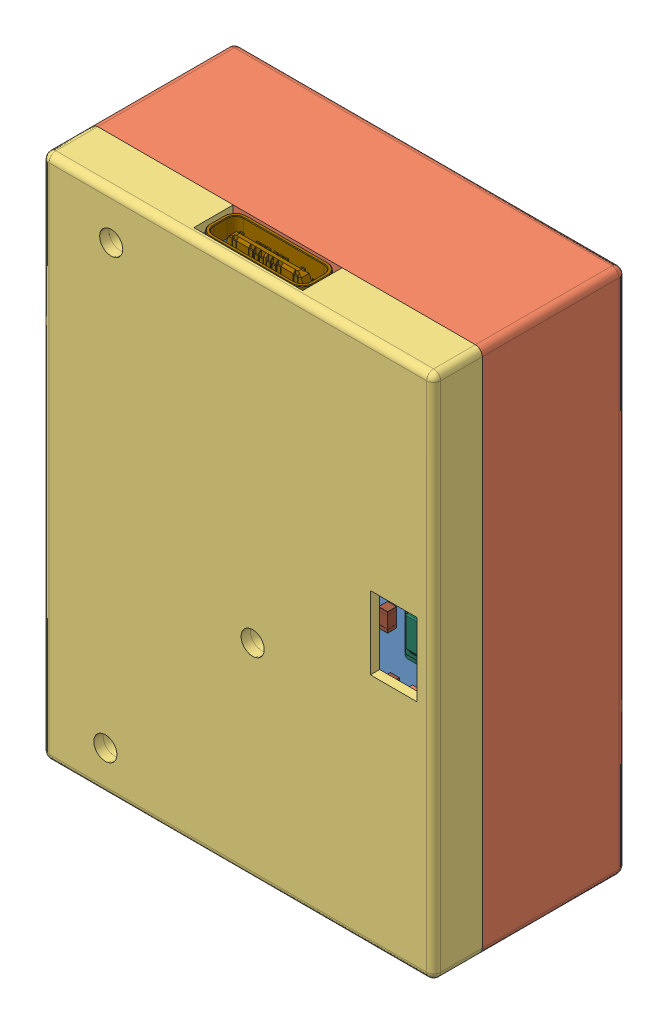
SolidWorks assembly 装配体v3.0, configuration 默认. Lengths in mm.
Overall size (33.77 45.37 16.59).
124 component instances, 21 part files, 8 mates.
Components (placement in the parent):
- 3D_主控_2025-09-16.step-1: 3D_主控_2025-09-16.step [默认] at (-99.2028 -82.7519 -1.9344) size (29.97 44.3 5.71)
  - U3~DFN-4_L1.5-W1.5-P0.8-TL-EP~DFN-4_L1.5-W1.5-P0.8~N7qM.step-1: U3~DFN-4_L1.5-W1.5-P0.8-TL-EP~DFN-4_L1.5-W1.5-P0.8~N7qM.step [默认] at (23.622 -32.2581 0) x (0 -1 0) z (0 0 -1) size (1.52 1.52 0.55)
    - DFN-4_L1.5-W1.5-P0.8-TL-EP~DFN-4_L1.5-W1.5-P0.8~N7qM.step-1: DFN-4_L1.5-W1.5-P0.8-TL-EP~DFN-4_L1.5-W1.5-P0.8~N7qM.step [默认] at origin size (1.52 1.52 0.55)
  - R1~R0603~R0603~N7qM.step-1: R1~R0603~R0603~N7qM.step [默认] at (25.6541 -14.224 1.5862) x (0 1 0) z (0 0 1) size (1.62 0.81 0.45)
    - R0603~R0603~N7qM.step-1: R0603~R0603~N7qM.step [默认] at origin size (1.62 0.81 0.45)
  - R1~R0603~R0603~N7qM.step-2: R1~R0603~R0603~N7qM.step [默认] at (23.241 -17.78 1.5862) size (1.62 0.81 0.45)
    - R0603~R0603~N7qM.step-1: R0603~R0603~N7qM.step [默认] at origin size (1.62 0.81 0.45)
  - R1~R0603~R0603~N7qM.step-3: R1~R0603~R0603~N7qM.step [默认] at (23.495 -34.7981 1.5862) x (0 -1 0) z (0 0 1) size (1.62 0.81 0.45)
    - R0603~R0603~N7qM.step-1: R0603~R0603~N7qM.step [默认] at origin size (1.62 0.81 0.45)
  - R1~R0603~R0603~N7qM.step-4: R1~R0603~R0603~N7qM.step [默认] at (27.5263 -28.0739 1.5862) x (0 1 0) z (0 0 1) size (1.62 0.81 0.45)
    - R0603~R0603~N7qM.step-1: R0603~R0603~N7qM.step [默认] at origin size (1.62 0.81 0.45)
  - R1~R0603~R0603~N7qM.step-5: R1~R0603~R0603~N7qM.step [默认] at (11.684 -10.668 1.5862) x (-1 0 0) z (0 0 1) size (1.62 0.81 0.45)
    - R0603~R0603~N7qM.step-1: R0603~R0603~N7qM.step [默认] at origin size (1.62 0.81 0.45)
  - R1~R0603~R0603~N7qM.step-6: R1~R0603~R0603~N7qM.step [默认] at (11.684 -9.144 1.5862) x (-1 0 0) z (0 0 1) size (1.62 0.81 0.45)
    - R0603~R0603~N7qM.step-1: R0603~R0603~N7qM.step [默认] at origin size (1.62 0.81 0.45)
  - R1~R0603~R0603~N7qM.step-7: R1~R0603~R0603~N7qM.step [默认] at (25.4001 -31.6231 1.5862) x (0 -1 0) z (0 0 1) size (1.62 0.81 0.45)
    - R0603~R0603~N7qM.step-1: R0603~R0603~N7qM.step [默认] at origin size (1.62 0.81 0.45)
  - R1~R0603~R0603~N7qM.step-8: R1~R0603~R0603~N7qM.step [默认] at (3.556 -9.398 1.5862) x (0 -1 0) z (0 0 1) size (1.62 0.81 0.45)
    - R0603~R0603~N7qM.step-1: R0603~R0603~N7qM.step [默认] at origin size (1.62 0.81 0.45)
  - R1~R0603~R0603~N7qM.step-9: R1~R0603~R0603~N7qM.step [默认] at (25.3867 -28.0538 1.5862) x (0 -1 0) z (0 0 1) size (1.62 0.81 0.45)
    - R0603~R0603~N7qM.step-1: R0603~R0603~N7qM.step [默认] at origin size (1.62 0.81 0.45)
  - R1~R0603~R0603~N7qM.step-10: R1~R0603~R0603~N7qM.step [默认] at (2.032 -14.859 1.5862) x (0 -1 0) z (0 0 1) size (1.62 0.81 0.45)
    - R0603~R0603~N7qM.step-1: R0603~R0603~N7qM.step [默认] at origin size (1.62 0.81 0.45)
  - R1~R0603~R0603~N7qM.step-11: R1~R0603~R0603~N7qM.step [默认] at (3.683 -14.859 1.5862) x (0 -1 0) z (0 0 1) size (1.62 0.81 0.45)
    - R0603~R0603~N7qM.step-1: R0603~R0603~N7qM.step [默认] at origin size (1.62 0.81 0.45)
  - R1~R0603~R0603~N7qM.step-12: R1~R0603~R0603~N7qM.step [默认] at (22.606 -5.969 1.5862) size (1.62 0.81 0.45)
    - R0603~R0603~N7qM.step-1: R0603~R0603~N7qM.step [默认] at origin size (1.62 0.81 0.45)
  - R1~R0603~R0603~N7qM.step-13: R1~R0603~R0603~N7qM.step [默认] at (22.606 -7.747 1.5862) size (1.62 0.81 0.45)
    - R0603~R0603~N7qM.step-1: R0603~R0603~N7qM.step [默认] at origin size (1.62 0.81 0.45)
  - R1~R0603~R0603~N7qM.step-14: R1~R0603~R0603~N7qM.step [默认] at (11.684 -13.081 1.5862) size (1.62 0.81 0.45)
    - R0603~R0603~N7qM.step-1: R0603~R0603~N7qM.step [默认] at origin size (1.62 0.81 0.45)
  - R1~R0603~R0603~N7qM.step-15: R1~R0603~R0603~N7qM.step [默认] at (24.384 -37.5921 0) x (-1 0 0) z (0 0 -1) size (1.62 0.81 0.45)
    - R0603~R0603~N7qM.step-1: R0603~R0603~N7qM.step [默认] at origin size (1.62 0.81 0.45)
  - R1~R0603~R0603~N7qM.step-16: R1~R0603~R0603~N7qM.step [默认] at (24.384 -39.4971 0) x (-1 0 0) z (0 0 -1) size (1.62 0.81 0.45)
    - R0603~R0603~N7qM.step-1: R0603~R0603~N7qM.step [默认] at origin size (1.62 0.81 0.45)
  - R1~R0603~R0603~N7qM.step-17: R1~R0603~R0603~N7qM.step [默认] at (5.969 -5.842 1.5862) size (1.62 0.81 0.45)
    - R0603~R0603~N7qM.step-1: R0603~R0603~N7qM.step [默认] at origin size (1.62 0.81 0.45)
  - R1~R0603~R0603~N7qM.step-18: R1~R0603~R0603~N7qM.step [默认] at (18.161 -30.8611 1.5862) x (0 -1 0) z (0 0 1) size (1.62 0.81 0.45)
    - R0603~R0603~N7qM.step-1: R0603~R0603~N7qM.step [默认] at origin size (1.62 0.81 0.45)
  - fin~LED_0603~LED-0603_G~N7qM.step-1: fin~LED_0603~LED-0603_G~N7qM.step [默认] at (26.1621 -7.747 1.5862) size (1.6 0.8 0.6)
    - LED_0603~LED-0603_G~N7qM.step-1: LED_0603~LED-0603_G~N7qM.step [默认] at origin size (1.6 0.8 0.6)
  - L1~L0603~L0603_L1.6-W0.8-H0.5_BEAD~N7qM.step-1: L1~L0603~L0603_L1.6-W0.8-H0.5_BEAD~N7qM.step [默认] at (9.144 -28.5751 1.5862) x (0 1 0) z (0 0 1) size (1.6 0.8 0.5)
    - L0603~L0603_L1.6-W0.8-H0.5_BEAD~N7qM.step-1: L0603~L0603_L1.6-W0.8-H0.5_BEAD~N7qM.step [默认] at origin size (1.6 0.8 0.5)
  - in~LED_0603~LED-0603_R~N7qM.step-1: in~LED_0603~LED-0603_R~N7qM.step [默认] at (27.5591 -31.6231 1.5862) x (0 1 0) z (0 0 1) size (1.49 0.75 0.56)
    - LED_0603~LED-0603_R~N7qM.step-1: LED_0603~LED-0603_R~N7qM.step [默认] at origin size (1.49 0.75 0.56)
  - in~LED_0603~LED-0603_R~N7qM.step-2: in~LED_0603~LED-0603_R~N7qM.step [默认] at (26.1621 -5.969 1.5862) size (1.49 0.75 0.56)
    - LED_0603~LED-0603_R~N7qM.step-1: LED_0603~LED-0603_R~N7qM.step [默认] at origin size (1.49 0.75 0.56)
  - U4~HLGA-10L_LPS22HBTR~HLGA-10L_L2.0-W2.0-H0.8-P0.5-LPS22HBTR~N7qM.step-1: U4~HLGA-10L_LPS22HBTR~HLGA-10L_L2.0-W2.0-H0.8-P0.5-LPS22HBTR~N7qM.step [默认] at (23.495 -28.4481 0) x (0 -1 0) z (0 0 -1) size (2 2 0.8)
    - HLGA-10L_LPS22HBTR~HLGA-10L_L2.0-W2.0-H0.8-P0.5-LPS22HBTR~N7qM.step-1: HLGA-10L_LPS22HBTR~HLGA-10L_L2.0-W2.0-H0.8-P0.5-LPS22HBTR~N7qM.step [默认] at origin size (2 2 0.8)
  - U5~DFN-6_L2.5-W2.5-P0.8-BL-EP~DFN-6_L2.5-W2.5-0.9-P0.8-BL-EP~N7qM.step-1: U5~DFN-6_L2.5-W2.5-P0.8-BL-EP~DFN-6_L2.5-W2.5-0.9-P0.8-BL-EP~N7qM.step [默认] at (27.3572 -31.423 0) x (-1 0 0) z (0 0 -1) size (2.47 2.47 0.92)
    - DFN-6_L2.5-W2.5-P0.8-BL-EP~DFN-6_L2.5-W2.5-0.9-P0.8-BL-EP~N7qM.step-1: DFN-6_L2.5-W2.5-P0.8-BL-EP~DFN-6_L2.5-W2.5-0.9-P0.8-BL-EP~N7qM.step [默认] at origin size (2.47 2.47 0.92)
  - BLECON~LED_0603~LED-0603_B~N7qM.step-1: BLECON~LED_0603~LED-0603_B~N7qM.step [默认] at (23.495 -31.7501 1.5862) x (0 -1 0) z (0 0 1) size (1.6 0.8 0.6)
    - LED_0603~LED-0603_B~N7qM.step-1: LED_0603~LED-0603_B~N7qM.step [默认] at origin size (1.6 0.8 0.6)
  - USB1~USB_ TYPE-C-6P~USB-SMD_U262-061N-4BVC11~N7qM.step-1: USB1~USB_ TYPE-C-6P~USB-SMD_U262-061N-4BVC11~N7qM.step [默认] at (14.224 -4.064 1.5862) x (-1 0 0) z (0 0 1) size (8.95 7.15 4.2)
    - USB_ TYPE-C-6P~USB-SMD_U262-061N-4BVC11~N7qM.step-1: USB_ TYPE-C-6P~USB-SMD_U262-061N-4BVC11~N7qM.step [默认] at origin size (8.95 7.15 4.2)
  - U2~SOT-23-3_L3.0-W1.7-P0.95-LS2.9-BR~SOT-23-3L_L2.9-W1.6-H1.1-LS2.8-P0.95~N7qM.step-1: U2~SOT-23-3_L3.0-W1.7-P0.95-LS2.9-BR~SOT-23-3L_L2.9-W1.6-H1.1-LS2.8-P0.95~N7qM.step [默认] at (17.018 -22.987 1.5862) x (0 1 0) z (0 0 1) size (2.8 2.9 1.1)
    - SOT-23-3_L2.9-W1.6-P1.90-LS2.8-BR~SOT-23-3L_L2.9-W1.6-H1.1-LS2.8-P0.95~N7qM.step-1: SOT-23-3_L2.9-W1.6-P1.90-LS2.8-BR~SOT-23-3L_L2.9-W1.6-H1.1-LS2.8-P0.95~N7qM.step [默认] at origin size (2.8 2.9 1.1)
  - U2~SOT-23-3_L3.0-W1.7-P0.95-LS2.9-BR~SOT-23-3L_L2.9-W1.6-H1.1-LS2.8-P0.95~N7qM.step-2: U2~SOT-23-3_L3.0-W1.7-P0.95-LS2.9-BR~SOT-23-3L_L2.9-W1.6-H1.1-LS2.8-P0.95~N7qM.step [默认] at (7.112 -23.622 1.5862) x (-1 0 0) z (0 0 1) size (2.8 2.9 1.1)
    - SOT-23-3_L2.9-W1.6-P1.90-LS2.8-BR~SOT-23-3L_L2.9-W1.6-H1.1-LS2.8-P0.95~N7qM.step-1: SOT-23-3_L2.9-W1.6-P1.90-LS2.8-BR~SOT-23-3L_L2.9-W1.6-H1.1-LS2.8-P0.95~N7qM.step [默认] at origin size (2.8 2.9 1.1)
  - C1~C0603~C0603_L1.6-W0.8-H0.8~N7qM.step-1: C1~C0603~C0603_L1.6-W0.8-H0.8~N7qM.step [默认] at (19.939 -30.8611 1.5862) x (0 1 0) z (0 0 1) size (1.6 0.8 0.8)
    - C0603~C0603_L1.6-W0.8-H0.8~N7qM.step-1: C0603~C0603_L1.6-W0.8-H0.8~N7qM.step [默认] at origin size (1.6 0.8 0.8)
  - C1~C0603~C0603_L1.6-W0.8-H0.8~N7qM.step-2: C1~C0603~C0603_L1.6-W0.8-H0.8~N7qM.step [默认] at (19.0465 -34.1595 1.5862) size (1.6 0.8 0.8)
    - C0603~C0603_L1.6-W0.8-H0.8~N7qM.step-1: C0603~C0603_L1.6-W0.8-H0.8~N7qM.step [默认] at origin size (1.6 0.8 0.8)
  - C1~C0603~C0603_L1.6-W0.8-H0.8~N7qM.step-3: C1~C0603~C0603_L1.6-W0.8-H0.8~N7qM.step [默认] at (19.0465 -35.9375 1.5862) size (1.6 0.8 0.8)
    - C0603~C0603_L1.6-W0.8-H0.8~N7qM.step-1: C0603~C0603_L1.6-W0.8-H0.8~N7qM.step [默认] at origin size (1.6 0.8 0.8)
  - C1~C0603~C0603_L1.6-W0.8-H0.8~N7qM.step-4: C1~C0603~C0603_L1.6-W0.8-H0.8~N7qM.step [默认] at (15.748 -35.306 1.5862) x (0 -1 0) z (0 0 1) size (1.6 0.8 0.8)
    - C0603~C0603_L1.6-W0.8-H0.8~N7qM.step-1: C0603~C0603_L1.6-W0.8-H0.8~N7qM.step [默认] at origin size (1.6 0.8 0.8)
  - C1~C0603~C0603_L1.6-W0.8-H0.8~N7qM.step-5: C1~C0603~C0603_L1.6-W0.8-H0.8~N7qM.step [默认] at (13.97 -35.306 1.5862) x (0 -1 0) z (0 0 1) size (1.6 0.8 0.8)
    - C0603~C0603_L1.6-W0.8-H0.8~N7qM.step-1: C0603~C0603_L1.6-W0.8-H0.8~N7qM.step [默认] at origin size (1.6 0.8 0.8)
  - C1~C0603~C0603_L1.6-W0.8-H0.8~N7qM.step-6: C1~C0603~C0603_L1.6-W0.8-H0.8~N7qM.step [默认] at (6.604 -18.669 1.5862) size (1.6 0.8 0.8)
    - C0603~C0603_L1.6-W0.8-H0.8~N7qM.step-1: C0603~C0603_L1.6-W0.8-H0.8~N7qM.step [默认] at origin size (1.6 0.8 0.8)
  - C1~C0603~C0603_L1.6-W0.8-H0.8~N7qM.step-7: C1~C0603~C0603_L1.6-W0.8-H0.8~N7qM.step [默认] at (6.604 -20.701 1.5862) size (1.6 0.8 0.8)
    - C0603~C0603_L1.6-W0.8-H0.8~N7qM.step-1: C0603~C0603_L1.6-W0.8-H0.8~N7qM.step [默认] at origin size (1.6 0.8 0.8)
  - C1~C0603~C0603_L1.6-W0.8-H0.8~N7qM.step-8: C1~C0603~C0603_L1.6-W0.8-H0.8~N7qM.step [默认] at (4.318 -23.622 1.5862) x (0 -1 0) z (0 0 1) size (1.6 0.8 0.8)
    - C0603~C0603_L1.6-W0.8-H0.8~N7qM.step-1: C0603~C0603_L1.6-W0.8-H0.8~N7qM.step [默认] at origin size (1.6 0.8 0.8)
  - C1~C0603~C0603_L1.6-W0.8-H0.8~N7qM.step-9: C1~C0603~C0603_L1.6-W0.8-H0.8~N7qM.step [默认] at (2.159 -23.622 1.5862) x (0 -1 0) z (0 0 1) size (1.6 0.8 0.8)
    - C0603~C0603_L1.6-W0.8-H0.8~N7qM.step-1: C0603~C0603_L1.6-W0.8-H0.8~N7qM.step [默认] at origin size (1.6 0.8 0.8)
  - C1~C0603~C0603_L1.6-W0.8-H0.8~N7qM.step-10: C1~C0603~C0603_L1.6-W0.8-H0.8~N7qM.step [默认] at (9.144 -28.5751 0) x (0 1 0) z (0 0 -1) size (1.6 0.8 0.8)
    - C0603~C0603_L1.6-W0.8-H0.8~N7qM.step-1: C0603~C0603_L1.6-W0.8-H0.8~N7qM.step [默认] at origin size (1.6 0.8 0.8)
  - C1~C0603~C0603_L1.6-W0.8-H0.8~N7qM.step-11: C1~C0603~C0603_L1.6-W0.8-H0.8~N7qM.step [默认] at (7.112 -32.5121 1.5862) x (0 -1 0) z (0 0 1) size (1.6 0.8 0.8)
    - C0603~C0603_L1.6-W0.8-H0.8~N7qM.step-1: C0603~C0603_L1.6-W0.8-H0.8~N7qM.step [默认] at origin size (1.6 0.8 0.8)
  - C1~C0603~C0603_L1.6-W0.8-H0.8~N7qM.step-12: C1~C0603~C0603_L1.6-W0.8-H0.8~N7qM.step [默认] at (11.049 -28.5751 0) x (0 1 0) z (0 0 -1) size (1.6 0.8 0.8)
    - C0603~C0603_L1.6-W0.8-H0.8~N7qM.step-1: C0603~C0603_L1.6-W0.8-H0.8~N7qM.step [默认] at origin size (1.6 0.8 0.8)
  - C1~C0603~C0603_L1.6-W0.8-H0.8~N7qM.step-13: C1~C0603~C0603_L1.6-W0.8-H0.8~N7qM.step [默认] at (8.89 -32.5121 1.5862) x (0 1 0) z (0 0 1) size (1.6 0.8 0.8)
    - C0603~C0603_L1.6-W0.8-H0.8~N7qM.step-1: C0603~C0603_L1.6-W0.8-H0.8~N7qM.step [默认] at origin size (1.6 0.8 0.8)
  - C1~C0603~C0603_L1.6-W0.8-H0.8~N7qM.step-14: C1~C0603~C0603_L1.6-W0.8-H0.8~N7qM.step [默认] at (23.368 -9.652 1.5862) size (1.6 0.8 0.8)
    - C0603~C0603_L1.6-W0.8-H0.8~N7qM.step-1: C0603~C0603_L1.6-W0.8-H0.8~N7qM.step [默认] at origin size (1.6 0.8 0.8)
  - C1~C0603~C0603_L1.6-W0.8-H0.8~N7qM.step-15: C1~C0603~C0603_L1.6-W0.8-H0.8~N7qM.step [默认] at (19.685 -22.86 1.5862) x (0 -1 0) z (0 0 1) size (1.6 0.8 0.8)
    - C0603~C0603_L1.6-W0.8-H0.8~N7qM.step-1: C0603~C0603_L1.6-W0.8-H0.8~N7qM.step [默认] at origin size (1.6 0.8 0.8)
  - C1~C0603~C0603_L1.6-W0.8-H0.8~N7qM.step-16: C1~C0603~C0603_L1.6-W0.8-H0.8~N7qM.step [默认] at (21.463 -22.86 1.5862) x (0 -1 0) z (0 0 1) size (1.6 0.8 0.8)
    - C0603~C0603_L1.6-W0.8-H0.8~N7qM.step-1: C0603~C0603_L1.6-W0.8-H0.8~N7qM.step [默认] at origin size (1.6 0.8 0.8)
  - C1~C0603~C0603_L1.6-W0.8-H0.8~N7qM.step-17: C1~C0603~C0603_L1.6-W0.8-H0.8~N7qM.step [默认] at (12.573 -22.86 1.5862) x (0 1 0) z (0 0 1) size (1.6 0.8 0.8)
    - C0603~C0603_L1.6-W0.8-H0.8~N7qM.step-1: C0603~C0603_L1.6-W0.8-H0.8~N7qM.step [默认] at origin size (1.6 0.8 0.8)
  - C1~C0603~C0603_L1.6-W0.8-H0.8~N7qM.step-18: C1~C0603~C0603_L1.6-W0.8-H0.8~N7qM.step [默认] at (14.351 -22.86 1.5862) x (0 1 0) z (0 0 1) size (1.6 0.8 0.8)
    - C0603~C0603_L1.6-W0.8-H0.8~N7qM.step-1: C0603~C0603_L1.6-W0.8-H0.8~N7qM.step [默认] at origin size (1.6 0.8 0.8)
  - C1~C0603~C0603_L1.6-W0.8-H0.8~N7qM.step-19: C1~C0603~C0603_L1.6-W0.8-H0.8~N7qM.step [默认] at (23.241 -22.86 1.5862) x (0 1 0) z (0 0 1) size (1.6 0.8 0.8)
    - C0603~C0603_L1.6-W0.8-H0.8~N7qM.step-1: C0603~C0603_L1.6-W0.8-H0.8~N7qM.step [默认] at origin size (1.6 0.8 0.8)
  - C1~C0603~C0603_L1.6-W0.8-H0.8~N7qM.step-20: C1~C0603~C0603_L1.6-W0.8-H0.8~N7qM.step [默认] at (6.985 -38.1001 0) x (0 1 0) z (0 0 -1) size (1.6 0.8 0.8)
    - C0603~C0603_L1.6-W0.8-H0.8~N7qM.step-1: C0603~C0603_L1.6-W0.8-H0.8~N7qM.step [默认] at origin size (1.6 0.8 0.8)
  - C1~C0603~C0603_L1.6-W0.8-H0.8~N7qM.step-21: C1~C0603~C0603_L1.6-W0.8-H0.8~N7qM.step [默认] at (10.414 -40.8941 0) x (1 0 0) z (0 0 -1) size (1.6 0.8 0.8)
    - C0603~C0603_L1.6-W0.8-H0.8~N7qM.step-1: C0603~C0603_L1.6-W0.8-H0.8~N7qM.step [默认] at origin size (1.6 0.8 0.8)
  - C1~C0603~C0603_L1.6-W0.8-H0.8~N7qM.step-22: C1~C0603~C0603_L1.6-W0.8-H0.8~N7qM.step [默认] at (23.4816 -28.0538 1.5862) x (0 1 0) z (0 0 1) size (1.6 0.8 0.8)
    - C0603~C0603_L1.6-W0.8-H0.8~N7qM.step-1: C0603~C0603_L1.6-W0.8-H0.8~N7qM.step [默认] at origin size (1.6 0.8 0.8)
  - C1~C0603~C0603_L1.6-W0.8-H0.8~N7qM.step-23: C1~C0603~C0603_L1.6-W0.8-H0.8~N7qM.step [默认] at (6.3659 -12.335 1.5862) size (1.6 0.8 0.8)
    - C0603~C0603_L1.6-W0.8-H0.8~N7qM.step-1: C0603~C0603_L1.6-W0.8-H0.8~N7qM.step [默认] at origin size (1.6 0.8 0.8)
  - C1~C0603~C0603_L1.6-W0.8-H0.8~N7qM.step-24: C1~C0603~C0603_L1.6-W0.8-H0.8~N7qM.step [默认] at (20.193 -30.3531 0) x (0 1 0) z (0 0 -1) size (1.6 0.8 0.8)
    - C0603~C0603_L1.6-W0.8-H0.8~N7qM.step-1: C0603~C0603_L1.6-W0.8-H0.8~N7qM.step [默认] at origin size (1.6 0.8 0.8)
  - U11~SOP-8_L4.9-W3.9-P1.27-LS6.0-BL-EP~SOP-8_L4.9-W3.9-H1.7-LS6.0-P1.30~N7qM.step-1: U11~SOP-8_L4.9-W3.9-P1.27-LS6.0-BL-EP~SOP-8_L4.9-W3.9-H1.7-LS6.0-P1.30~N7qM.step [默认] at (17.526 -12.319 1.5862) size (4.81 6 1.72)
    - SOP-8_L4.9-W3.9-P1.27-LS6.0-BL-EP~SOP-8_L4.9-W3.9-H1.7-LS6.0-P1.30~N7qM.step-1: SOP-8_L4.9-W3.9-P1.27-LS6.0-BL-EP~SOP-8_L4.9-W3.9-H1.7-LS6.0-P1.30~N7qM.step [默认] at origin size (4.81 6 1.72)
  - 32MHz~OSC-SMD_4P-L3.2-W2.5-BL~OSC-SMD_4P-L3.2-W2.5-H1.0~N7qM.step-1: 32MHz~OSC-SMD_4P-L3.2-W2.5-BL~OSC-SMD_4P-L3.2-W2.5-H1.0~N7qM.step [默认] at (10.033 -38.2271 0) x (1 0 0) z (0 0 -1) size (3.2 2.5 0.81)
    - OSC-SMD_4P-L3.2-W2.5-BL~OSC-SMD_4P-L3.2-W2.5-H1.0~N7qM.step-1: OSC-SMD_4P-L3.2-W2.5-BL~OSC-SMD_4P-L3.2-W2.5-H1.0~N7qM.step [默认] at origin size (3.2 2.5 0.81)
  - U6~qfn-28_l4.0-w4.0-p0.40-bl-ep2.7~QFN-28_L4.0-W4.0-P0.40-BL-EP2.7~N7qM.step-1: U6~qfn-28_l4.0-w4.0-p0.40-bl-ep2.7~QFN-28_L4.0-W4.0-P0.40-BL-EP2.7~N7qM.step [默认] at (10.0253 -32.8188 0) x (1 0 0) z (0 0 -1) size (4.02 4.02 0.76)
    - qfn-28_l4.0-w4.0-p0.40-bl-ep2.7~QFN-28_L4.0-W4.0-P0.40-BL-EP2.7~N7qM.step-1: qfn-28_l4.0-w4.0-p0.40-bl-ep2.7~QFN-28_L4.0-W4.0-P0.40-BL-EP2.7~N7qM.step [默认] at origin size (4.02 4.02 0.76)
  - SW2~Key_SMD_3.6x6.1x2.5~KEY-SMD_2P-L6.0-W3.6-H2.5-LS8.0 COPY~N7qM.step-1: SW2~Key_SMD_3.6x6.1x2.5~KEY-SMD_2P-L6.0-W3.6-H2.5-LS8.0 COPY~N7qM.step [默认] at (27.5591 -20.955 1.5862) x (0 -1 0) z (0 0 1) size (7.9 3.6 2.6)
    - Key_SMD_3.6x6.1x2.5~KEY-SMD_2P-L6.0-W3.6-H2.5-LS8.0 COPY~N7qM.step-1: Key_SMD_3.6x6.1x2.5~KEY-SMD_2P-L6.0-W3.6-H2.5-LS8.0 COPY~N7qM.step [默认] at origin size (7.9 3.6 2.6)
  - U1~UFQFPN-32_L5.0-W5.0-P0.50-BL-EP~UFQFPN-32_L5.0-W5.0-H0.6-P0.50~N7qM.step-1: U1~UFQFPN-32_L5.0-W5.0-P0.50-BL-EP~UFQFPN-32_L5.0-W5.0-H0.6-P0.50~N7qM.step [默认] at (16.256 -32.7661 0) x (0 -1 0) z (0 0 -1) size (5 5 0.61)
    - UFQFPN-32_L5.0-W5.0-P0.50-BL-EP~UFQFPN-32_L5.0-W5.0-H0.6-P0.50~N7qM.step-1: UFQFPN-32_L5.0-W5.0-P0.50-BL-EP~UFQFPN-32_L5.0-W5.0-H0.6-P0.50~N7qM.step [默认] at origin size (5 5 0.61)
  - L3~IND-SMD_L2.5-W2.0_SWPA2520~IND-SMD_L2.5-W2.0-H1.2-252012~N7qM.step-1: L3~IND-SMD_L2.5-W2.0_SWPA2520~IND-SMD_L2.5-W2.0-H1.2-252012~N7qM.step [默认] at (9.779 -17.018 1.5862) x (0 -1 0) z (0 0 1) size (2.52 2 1.21)
    - IND-SMD_L2.5-W2.0_SWPA2520~IND-SMD_L2.5-W2.0-H1.2-252012~N7qM.step-1: IND-SMD_L2.5-W2.0_SWPA2520~IND-SMD_L2.5-W2.0-H1.2-252012~N7qM.step [默认] at origin size (2.52 2 1.21)
  - U12~SOT-23-5_L3.0-W1.7-P0.95-LS2.8-BR~SOT-23-5_L2.9-W1.6-H1.1-LS2.8-P0.95~N7qM.step-1: U12~SOT-23-5_L3.0-W1.7-P0.95-LS2.8-BR~SOT-23-5_L2.9-W1.6-H1.1-LS2.8-P0.95~N7qM.step [默认] at (6.096 -8.763 1.5862) x (0 1 0) z (0 0 1) size (2.89 2.78 1.2)
    - SOT-23-5_L3.0-W1.7-P0.95-LS2.8-BR~SOT-23-5_L2.9-W1.6-H1.1-LS2.8-P0.95~N7qM.step-1: SOT-23-5_L3.0-W1.7-P0.95-LS2.8-BR~SOT-23-5_L2.9-W1.6-H1.1-LS2.8-P0.95~N7qM.step [默认] at origin size (2.89 2.78 1.2)
  - Board~N7qM.step-1: Board~N7qM.step [默认] at origin size (29.97 43.57 1.59)
- 零件40^装配体v3.0-1: 零件40^装配体v3.0 [默认] at (-99.2028 -82.7519 -1.9344) x (-1 0 0) z (0 0 -1) size (33.77 45.37 12.39) (virtual)
- 零件41^装配体v3.0-2: 零件41^装配体v3.0 [默认] at (-99.2028 -82.7519 -0.3482) size (33.77 45.37 4.2) (virtual)
Mates (geometry in assembly coordinates):
- 在位2: in place: plane of 3D_主控_2025-09-16.step-1/Board~N7qM.step-1 through (-84.0758 -104.552 -1.9344) normal (0 0 -1); plane of ? through (0 0 -1.9344) normal (0 0 -1); moOrthogonalPlaneRef_w of 3D_主控_2025-09-16.step-1/Board~N7qM.step-1 through (-84.0758 -104.552 -1.9344) normal (0 0 -1); plane of ? through (0 0 -1.9344) normal (0 1 0); plane of 3D_主控_2025-09-16.step-1/Board~N7qM.step-1 through (-84.0758 -104.552 -1.9344) normal (0 0 -1); plane of ? through (0 0 -1.9344) normal (-1 0 0); plane of 3D_主控_2025-09-16.step-1/Board~N7qM.step-1 through (-84.0758 -104.552 -1.9344) normal (0 0 -1); unknown of 零件40^装配体v3.0-1
- 重合4: coincident aligned: plane of 3D_主控_2025-09-16.step-1/Board~N7qM.step-1; plane of 零件40^装配体v3.0-1
- 重合5: coincident aligned: moOrthogonalPlaneRef_w of 3D_主控_2025-09-16.step-1/Board~N7qM.step-1 through (-99.2028 -82.7519 -1.9344) normal (0 1 0); plane of 零件40^装配体v3.0-1 through (-99.2028 -82.7519 -1.9344) normal (0 1 0)
- 重合6: coincident anti-aligned: moOrthogonalPlaneRef_w of 3D_主控_2025-09-16.step-1/Board~N7qM.step-1 through (-99.2028 -82.7519 -1.9344) normal (1 0 0); plane of 零件40^装配体v3.0-1 through (-99.2028 -82.7519 -1.9344) normal (-1 0 0)
- 在位4: in place: plane of 3D_主控_2025-09-16.step-1/Board~N7qM.step-1 through (-84.0758 -104.552 -0.3482) normal (0 0 1); plane of ? through (0 0 -0.3482) normal (0 0 1); plane of 3D_主控_2025-09-16.step-1/Board~N7qM.step-1 through (-84.0758 -104.552 -0.3482) normal (0 0 1); plane of ? through (0 0 -0.3482) normal (0 1 0); plane of 3D_主控_2025-09-16.step-1/Board~N7qM.step-1 through (-84.0758 -104.552 -0.3482) normal (0 0 1); plane of ? through (0 0 -0.3482) normal (1 0 0); plane of 3D_主控_2025-09-16.step-1/Board~N7qM.step-1 through (-84.0758 -104.552 -0.3482) normal (0 0 1); unknown of 零件41^装配体v3.0-2
- 重合4: coincident aligned: plane of 3D_主控_2025-09-16.step-1/Board~N7qM.step-1; plane of 零件41^装配体v3.0-2
- 重合5: coincident aligned: moOrthogonalPlaneRef_w of 3D_主控_2025-09-16.step-1/Board~N7qM.step-1 through (-99.2028 -82.7519 -0.3482) normal (0 1 0); plane of 零件41^装配体v3.0-2 through (-99.2028 -82.7519 -0.3482) normal (0 1 0)
- 重合6: coincident anti-aligned: moOrthogonalPlaneRef_w of 3D_主控_2025-09-16.step-1/Board~N7qM.step-1 through (-99.2028 -82.7519 -0.3482) normal (-1 0 0); plane of 零件41^装配体v3.0-2 through (-99.2028 -82.7519 -0.3482) normal (1 0 0)
